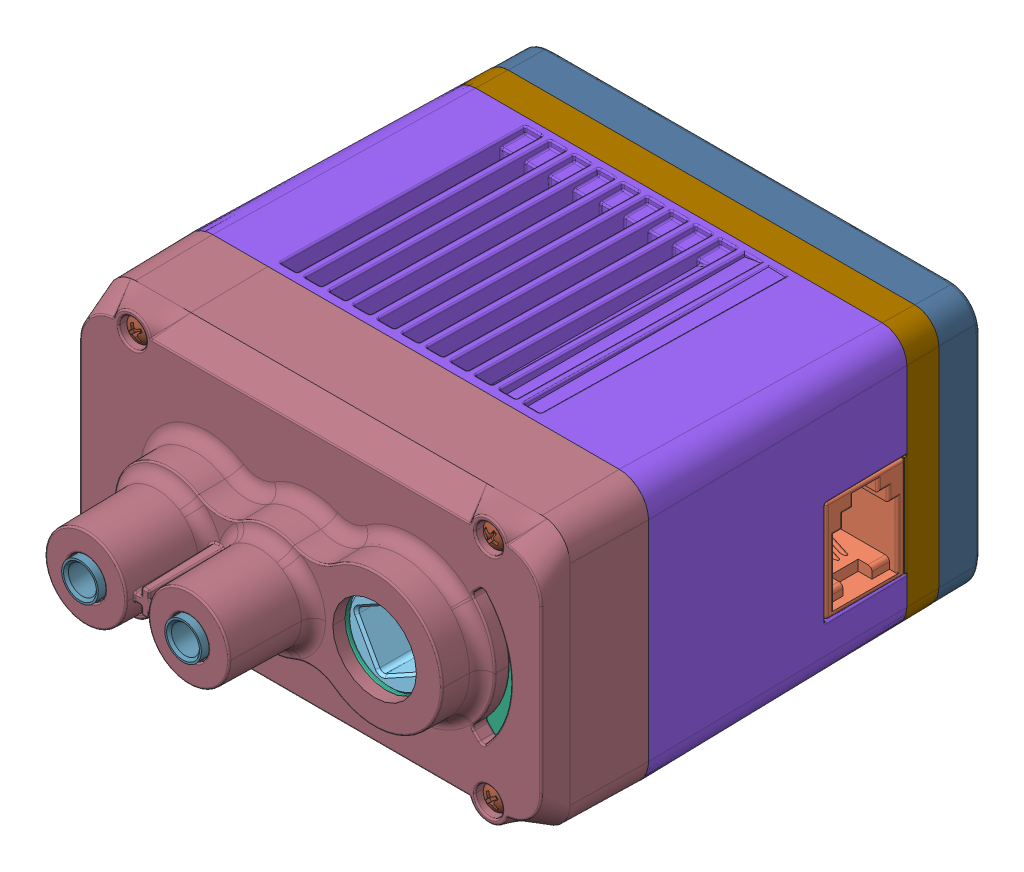
SolidWorks assembly V5 Smart Motor (276-4840) 2, configuration Default. Lengths in mm.
Overall size (59.01 35.33 72.31).
26 component instances, 15 part files, 0 mates.
Components (placement in the parent):
- V5 Smart Motor (276-4840) 2.step-1: V5 Smart Motor (276-4840) 2.step [Default] at origin size (59.01 35.33 72.31)
  - 276-4840-900 Rev6_Instruction.step-1: 276-4840-900 Rev6_Instruction.step [Default] at (-14.3 0 -17.2) size (52.79 15.94 38.15)
    - 276-4840-901 Rev6.step-1: 276-4840-901 Rev6.step [Default] at (10.75 -10.05 17.8) x (-1 0 0) z (0 0 1) size (49.9 1.6 38.15)
    - 276-4840-902 Rev2.step-1: 276-4840-902 Rev2.step [Default] at (31.25 -9.25 6.2) x (0 0 -1) z (0 -1 0) size (10.35 11.39 15.94)
    - 276-4840-022 Rev4.step-1: 276-4840-022 Rev4.step [Default] at (31.25 -9.25 6.2) x (0 0 -1) z (1 0 0) size (10.26 9.1 5.51)
  - 276-4840-110 Rev10_Instruction.step-1: 276-4840-110 Rev10_Instruction.step [Default] at (12.7 0 14.7) size (35.33 35.33 31.1)
    - 276-4840-061 Rev7_Ring_Gear_Fixed01 .6 Rev3.step-1: 276-4840-061 Rev7_Ring_Gear_Fixed01 .6 Rev3.step [Default] at origin size (28.79 28.39 24.6)
    - 276-4840-018 Rev6.step-1: 276-4840-018 Rev6.step [Default] at (0 0 6.7) x (-0.483174 0.875524 0) z (0 0 1) size (26 26 12.3)
    - 276-4840-059 Rev2.step-1: 276-4840-059 Rev2.step [Default] at (0 0 10.3) size (28.4 28.4 8.5)
    - 276-4840-062 Rev1.step-1: 276-4840-062 Rev1.step [Default] at (-12.1353 8.8168 12.3) x (0.956835 -0.290632 0) z (-0.290632 -0.956835 0) size (3.2 6.56 3.2)
    - 276-4840-062 Rev1.step-2: 276-4840-062 Rev1.step [Default] at (12.1353 8.8168 12.3) x (0.978427 0.206591 0) z (0.206591 -0.978427 0) size (3.2 6.56 3.2)
    - 276-4840-062 Rev1.step-3: 276-4840-062 Rev1.step [Default] at (-12.1353 -8.8168 12.3) x (0.72563 0.688086 0) z (0.688086 -0.72563 0) size (3.2 6.56 3.2)
  - 276-4840-001 Rev38.step-1: 276-4840-001 Rev38.step [Default] at origin size (57.3 33 46.9)
  - 276-4840-005 Rev27.step-1: 276-4840-005 Rev27.step [Default] at (0 0 -17.95) size (56.17 31.87 12.9)
  - 276-4840-004 Rev16.step-1: 276-4840-004 Rev16.step [Default] at (0 0 -19.2) size (56.01 31.71 9.21)
  - 276-4840-015 Rev7.step-1: 276-4840-015 Rev7.step [Default] at (-21.95 14 27.9) x (-0.85131 -0.524663 0) z (-0.524663 0.85131 0) size (3.2 17.55 3.2)
  - 276-4840-015 Rev7.step-2: 276-4840-015 Rev7.step [Default] at (21.95 -14 27.9) x (-0.777574 -0.628792 0) z (-0.628792 0.777574 0) size (3.2 17.55 3.2)
  - 276-4840-015 Rev7.step-3: 276-4840-015 Rev7.step [Default] at (21.95 14 27.9) x (0.476859 0.87898 0) z (0.87898 -0.476859 0) size (3.2 17.55 3.2)
  - 276-4840-009 Rev3.step-1: 276-4840-009 Rev3.step [Default] at (25.45 13.5 15.7) x (0.19987 -0.979823 0) z (-0.979823 -0.19987 0) size (3.4 41.31 4.34)
  - 276-4840-009 Rev3.step-2: 276-4840-009 Rev3.step [Default] at (-25.45 -13.5 15.7) x (-0.998855 0.047836 0) z (0.047836 0.998855 0) size (3.4 41.31 4.34)
  - 276-4840-009 Rev3.step-3: 276-4840-009 Rev3.step [Default] at (25.45 -13.5 15.7) x (-0.975374 0.220559 0) z (0.220559 0.975374 0) size (3.4 41.31 4.34)
  - 276-4840-009 Rev3.step-4: 276-4840-009 Rev3.step [Default] at (-25.45 13.5 15.7) x (-0.922256 0.38658 0) z (0.38658 0.922256 0) size (3.4 41.31 4.34)
  - 276-4840-003 Rev27.step-1: 276-4840-003 Rev27.step [Default] at (0 0 16.2) size (57.3 33 28.01)
  - 276-4840-043 Rev8.step-1: 276-4840-043 Rev8.step [Default] at (-12.7 0 36.2) x (-0.5 -0.866025 0) z (-0.866025 0.5 0) size (6.3 15.2 7.21)
  - 276-4840-043 Rev8.step-2: 276-4840-043 Rev8.step [Default] at (0 0 36.2) x (-0.5 -0.866025 0) z (-0.866025 0.5 0) size (6.3 15.2 7.21)
  - 276-4840-025 Rev19.step-1: 276-4840-025 Rev19.step [Default] at (12.7 0 -22.63) x (-0.993315 0.115437 0) z (0 0 1) size (14.82 14.83 35.18)
